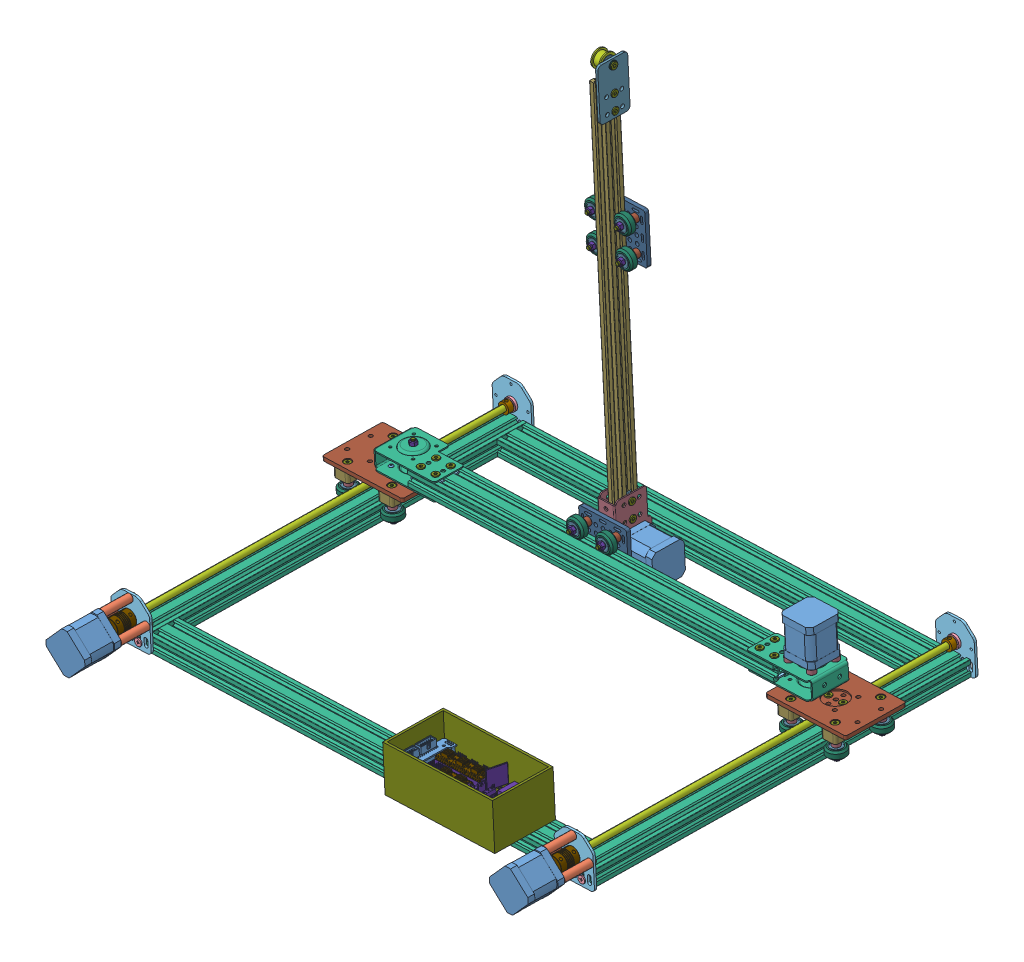
SolidWorks assembly manipulator2, configuration 預設. Lengths in mm. (continued)
Components (placement in the parent): (continued)
- Y-1: Y [Default] at (-55.2828 466.9625 1561.8962) x (0.061515 -0.998106 -0.000537) z (0.998106 0.061515 -0.00018) size (96.36 65.23 599.86) (flexible) (continued)
  - small plate-2: small plate [預設] at (444.4195 1082.4526 226.1786) x (0.999761 -0.019668 -0.009529) z (0.009662 0.00665 0.999931) size (65.63 34.48 65.67) (continued)
    - small wheel-5: small wheel [預設] at (-0.6906 23.95 24.7704) x (-0.019681 0.99952 0.023908) z (0.000235 -0.023908 0.999714) size (11 23.9 23.9) (continued)
      - Ball Bearing 5 x 16 x 5-2: Ball Bearing 5 x 16 x 5 [Default] at (-5.0567 -11.3534 -2.7479) size (5 16 16)
      - Solid V Wheel-2: Solid V Wheel [Default] at (-8.0567 -11.3534 -2.7479) size (10.2 23.9 23.9)
      - Ball Bearing 5 x 16 x 5-3: Ball Bearing 5 x 16 x 5 [Default] at (-11.0567 -11.3534 -2.7479) size (5 16 16)
    - small wheel-6: small wheel [預設] at (-40.6828 23.1636 24.7264) x (-0.019681 0.99952 0.023908) z (0.000235 -0.023908 0.999714) size (11 23.9 23.9)
      - Ball Bearing 5 x 16 x 5-2: Ball Bearing 5 x 16 x 5 [Default] at (-5.0567 -11.3534 -2.7479) size (5 16 16)
      - Solid V Wheel-2: Solid V Wheel [Default] at (-8.0567 -11.3534 -2.7479) size (10.2 23.9 23.9)
      - Ball Bearing 5 x 16 x 5-3: Ball Bearing 5 x 16 x 5 [Default] at (-11.0567 -11.3534 -2.7479) size (5 16 16)
    - Aluminum Spacer 9mm-1: Aluminum Spacer 9mm [Default] at (-29.3072 19.9403 61.9094) x (0.999806 0.019681 0.000235) z (-0.019681 0.99952 0.023908) size (10 10 9)
    - Aluminum Spacer 9mm-2: Aluminum Spacer 9mm [Default] at (10.6851 20.7267 61.9534) x (0.999806 0.019681 0.000235) z (-0.019681 0.99952 0.023908) size (10 10 9)
    - Aluminum Spacer 9mm-3: Aluminum Spacer 9mm [Default] at (-29.282 20.8973 21.9208) x (0.999806 0.019681 0.000235) z (-0.019681 0.99952 0.023908) size (10 10 9)
    - Aluminum Spacer 9mm-4: Aluminum Spacer 9mm [Default] at (10.7103 21.6837 21.9648) x (0.999806 0.019681 0.000235) z (-0.019681 0.99952 0.023908) size (10 10 9)
    - Low Profile Screw M5-7: Low Profile Screw M5 [M5 x 30] at (-28.9529 1.949 61.479) x (0.019681 -0.99952 -0.023908) z (0.000235 -0.023908 0.999714) size (31.62 9 9)
    - Low Profile Screw M5-8: Low Profile Screw M5 [M5 x 30] at (-28.9277 2.906 21.4905) x (0.019681 -0.99952 -0.023908) z (0.000235 -0.023908 0.999714) size (31.62 9 9)
    - Low Profile Screw M5-9: Low Profile Screw M5 [M5 x 30] at (11.0393 2.7354 61.523) x (0.019681 -0.99952 -0.023908) z (0.000235 -0.023908 0.999714) size (31.62 9 9)
    - Low Profile Screw M5-10: Low Profile Screw M5 [M5 x 30] at (11.0645 3.6924 21.5345) x (0.019681 -0.99952 -0.023908) z (0.000235 -0.023908 0.999714) size (31.62 9 9)
    - Nylon Insert Lock Nut M5-6: Nylon Insert Lock Nut M5 [Default] at (-29.0655 9.9026 21.6579) x (0.192329 -0.019681 0.981133) z (0.981133 0.023908 -0.191849) size (8 5 9.24)
    - Nylon Insert Lock Nut M5-7: Nylon Insert Lock Nut M5 [Default] at (-29.0907 8.9456 61.6464) x (0.192329 -0.019681 0.981133) z (0.981133 0.023908 -0.191849) size (8 5 9.24)
    - Nylon Insert Lock Nut M5-9: Nylon Insert Lock Nut M5 [Default] at (10.9016 9.732 61.6904) x (0.192329 -0.019681 0.981133) z (0.981133 0.023908 -0.191849) size (8 5 9.24)
    - Nylon Insert Lock Nut M5-10: Nylon Insert Lock Nut M5 [Default] at (10.9268 10.689 21.7018) x (0.192329 -0.019681 0.981133) z (0.981133 0.023908 -0.191849) size (8 5 9.24)
- X-1: X [Default] at (377.0186 755.9985 711.7917) x (-0.998451 -0.05295 -0.017075) z (0.052967 -0.998596 -0.000534) size (92.45 47.68 584.07) (flexible)
  - Double Tee Nut-1: Double Tee Nut [Default] at (171.529 282.1788 684.0965) x (0 0 -1) z (1 0 0) size (36.88 10 3)
  - Double Tee Nut-2: Double Tee Nut [Default] at (171.529 282.1788 220.9765) x (0 0 -1) z (1 0 0) size (36.88 10 3)
  - Low Profile Screw M5-13: Low Profile Screw M5 [M5 x 25] at (190.729 287.1788 160.7465) size (26.62 9 9)
  - Nylon Insert Lock Nut M5-4: Nylon Insert Lock Nut M5 [Default] at (185.829 287.1788 160.7465) x (0 -1 0) z (0 0 1) size (8 5 9.24)
  - Low Profile Screw M5-14: Low Profile Screw M5 [M5 x 8] at (174.729 287.1788 192.5365) size (9.62 9 9)
  - Low Profile Screw M5-15: Low Profile Screw M5 [M5 x 8] at (174.729 287.1788 212.5365) size (9.62 9 9)
  - Button Head Socket Cap Screw M3-1: Button Head Socket Cap Screw M3 [M3 x 8] at (161.729 302.6788 691.1565) x (-1 0 0) z (0 0.924225 0.381849) size (9.72 5.7 5.7)
  - Button Head Socket Cap Screw M3-3: Button Head Socket Cap Screw M3 [M3 x 8] at (161.729 302.6788 722.1565) x (-1 0 0) z (0 0.924225 0.381849) size (9.72 5.7 5.7)
  - Button Head Socket Cap Screw M3-4: Button Head Socket Cap Screw M3 [M3 x 8] at (161.729 271.6788 722.1565) x (-1 0 0) z (0 0.924225 0.381849) size (9.72 5.7 5.7)
  - Button Head Socket Cap Screw M3-5: Button Head Socket Cap Screw M3 [M3 x 8] at (161.729 271.6788 691.1565) x (-1 0 0) z (0 0.924225 0.381849) size (9.72 5.7 5.7)
  - Low Profile Screw M5-16: Low Profile Screw M5 [M5 x 8] at (176.129 287.1788 655.6565) size (9.62 9 9)
  - Low Profile Screw M5-17: Low Profile Screw M5 [M5 x 8] at (176.129 287.1788 675.6565) size (9.62 9 9)
  - Low Profile Screw M5-18: Low Profile Screw M5 [M5 x 8] at (183.329 287.1788 675.6565) x (-1 0 0) z (0 0.924225 0.381849) size (9.62 9 9)
  - Low Profile Screw M5-19: Low Profile Screw M5 [M5 x 8] at (183.329 287.1788 655.6565) x (-1 0 0) z (0 0.924225 0.381849) size (9.62 9 9)
  - Nema 17 Stepper Motor-1: Nema 17 Stepper Motor [Default] at (168.129 287.1788 706.6565) x (0 0 -1) z (1 0 0) size (42.42 42.42 72)
  - GT2 Timing Pulley 30 Tooth-1: GT2 Timing Pulley 30 Tooth [Default] at (191.729 287.1788 706.6565) x (-1 0 0) z (0 0.993409 -0.11462) size (17.5 22 22)
  - Smooth Idler-1: Smooth Idler [Default] at (179.279 287.1788 160.7465) x (-1 0 0) z (0 0.430653 -0.902518) size (13.1 22 22)
    - Smooth Idler Pulley Wheel-1: Smooth Idler Pulley Wheel [Default] at origin size (12.7 22 22)
    - Ball Bearing 5 x 16 x 5-1: Ball Bearing 5 x 16 x 5 [Default] at (4.05 0 0) x (1 0 0) z (0 0.954651 0.297727) size (5 16 16)
    - Ball Bearing 5 x 16 x 5-2: Ball Bearing 5 x 16 x 5 [Default] at (-4.05 0 0) x (1 0 0) z (0 0.976216 -0.216802) size (5 16 16)
    - Nylon Spacer 0.125in-1: Nylon Spacer 0.125in [Default] at (-1.625 0 0) x (0 -0.24187 -0.970309) z (0 -0.970309 0.24187) size (7.94 3.17 7.94)
  - V-Slot 20x20x500 Linear Rail-1: V-Slot 20x20x500 Linear Rail [Default] at (179.729 287.1788 184.0965) size (20 20 500)
  - small plate-1: small plate [預設] at (188.6703 270.6911 316.0744) x (0.999806 -0.019681 -0.000629) z (0.0011 0.023908 0.999714) size (65.63 34.48 65.67)
    - small wheel-3: small wheel [預設] at (-0.7158 22.993 64.759) x (-0.019681 0.99952 0.023908) z (0.000235 -0.023908 0.999714) size (11 23.9 23.9)
      - Ball Bearing 5 x 16 x 5-2: Ball Bearing 5 x 16 x 5 [Default] at (-5.0567 -11.3534 -2.7479) size (5 16 16)
      - Solid V Wheel-2: Solid V Wheel [Default] at (-8.0567 -11.3534 -2.7479) size (10.2 23.9 23.9)
      - Ball Bearing 5 x 16 x 5-3: Ball Bearing 5 x 16 x 5 [Default] at (-11.0567 -11.3534 -2.7479) size (5 16 16)
    - small wheel-4: small wheel [預設] at (-40.708 22.2066 64.715) x (-0.019681 0.99952 0.023908) z (0.000235 -0.023908 0.999714) size (11 23.9 23.9)
      - Ball Bearing 5 x 16 x 5-2: Ball Bearing 5 x 16 x 5 [Default] at (-5.0567 -11.3534 -2.7479) size (5 16 16)
      - Solid V Wheel-2: Solid V Wheel [Default] at (-8.0567 -11.3534 -2.7479) size (10.2 23.9 23.9)
      - Ball Bearing 5 x 16 x 5-3: Ball Bearing 5 x 16 x 5 [Default] at (-11.0567 -11.3534 -2.7479) size (5 16 16)
    - V-Slot Gantry Plate 20mm 2-1: V-Slot Gantry Plate 20mm 2 [Default] at (-9.4756 29.8077 42.1523) x (0.999806 0.01966 0.0011) z (-0.000629 -0.023925 0.999714) size (65.5 5 65.5)
    - small wheel-5: small wheel [預設] at (-0.6906 23.95 24.7704) x (-0.019681 0.99952 0.023908) z (0.000235 -0.023908 0.999714) size (11 23.9 23.9)
      - Ball Bearing 5 x 16 x 5-2: Ball Bearing 5 x 16 x 5 [Default] at (-5.0567 -11.3534 -2.7479) size (5 16 16)
      - Solid V Wheel-2: Solid V Wheel [Default] at (-8.0567 -11.3534 -2.7479) size (10.2 23.9 23.9)
      - Ball Bearing 5 x 16 x 5-3: Ball Bearing 5 x 16 x 5 [Default] at (-11.0567 -11.3534 -2.7479) size (5 16 16)
    - small wheel-6: small wheel [預設] at (-40.6828 23.1636 24.7264) x (-0.019681 0.99952 0.023908) z (0.000235 -0.023908 0.999714) size (11 23.9 23.9)
      - Ball Bearing 5 x 16 x 5-2: Ball Bearing 5 x 16 x 5 [Default] at (-5.0567 -11.3534 -2.7479) size (5 16 16)
      - Solid V Wheel-2: Solid V Wheel [Default] at (-8.0567 -11.3534 -2.7479) size (10.2 23.9 23.9)
      - Ball Bearing 5 x 16 x 5-3: Ball Bearing 5 x 16 x 5 [Default] at (-11.0567 -11.3534 -2.7479) size (5 16 16)
    - Aluminum Spacer 9mm-1: Aluminum Spacer 9mm [Default] at (-29.3072 19.9403 61.9094) x (0.999806 0.019681 0.000235) z (-0.019681 0.99952 0.023908) size (10 10 9)
    - Aluminum Spacer 9mm-2: Aluminum Spacer 9mm [Default] at (10.6851 20.7267 61.9534) x (0.999806 0.019681 0.000235) z (-0.019681 0.99952 0.023908) size (10 10 9)
    - Aluminum Spacer 9mm-3: Aluminum Spacer 9mm [Default] at (-29.282 20.8973 21.9208) x (0.999806 0.019681 0.000235) z (-0.019681 0.99952 0.023908) size (10 10 9)
    - Aluminum Spacer 9mm-4: Aluminum Spacer 9mm [Default] at (10.7103 21.6837 21.9648) x (0.999806 0.019681 0.000235) z (-0.019681 0.99952 0.023908) size (10 10 9)
    - Low Profile Screw M5-7: Low Profile Screw M5 [M5 x 30] at (-28.9529 1.949 61.479) x (0.019681 -0.99952 -0.023908) z (0.000235 -0.023908 0.999714) size (31.62 9 9)
    - Low Profile Screw M5-8: Low Profile Screw M5 [M5 x 30] at (-28.9277 2.906 21.4905) x (0.019681 -0.99952 -0.023908) z (0.000235 -0.023908 0.999714) size (31.62 9 9)
    - Low Profile Screw M5-9: Low Profile Screw M5 [M5 x 30] at (11.0393 2.7354 61.523) x (0.019681 -0.99952 -0.023908) z (0.000235 -0.023908 0.999714) size (31.62 9 9)
    - Low Profile Screw M5-10: Low Profile Screw M5 [M5 x 30] at (11.0645 3.6924 21.5345) x (0.019681 -0.99952 -0.023908) z (0.000235 -0.023908 0.999714) size (31.62 9 9)
    - Nylon Insert Lock Nut M5-6: Nylon Insert Lock Nut M5 [Default] at (-29.0655 9.9026 21.6579) x (0.192329 -0.019681 0.981133) z (0.981133 0.023908 -0.191849) size (8 5 9.24)
    - Nylon Insert Lock Nut M5-7: Nylon Insert Lock Nut M5 [Default] at (-29.0907 8.9456 61.6464) x (0.192329 -0.019681 0.981133) z (0.981133 0.023908 -0.191849) size (8 5 9.24)
    - Nylon Insert Lock Nut M5-9: Nylon Insert Lock Nut M5 [Default] at (10.9016 9.732 61.6904) x (0.192329 -0.019681 0.981133) z (0.981133 0.023908 -0.191849) size (8 5 9.24)
    - Nylon Insert Lock Nut M5-10: Nylon Insert Lock Nut M5 [Default] at (10.9268 10.689 21.7018) x (0.192329 -0.019681 0.981133) z (0.981133 0.023908 -0.191849) size (8 5 9.24)
  - Actuator End Mount 2-2: Actuator End Mount 2 [Default] at (149.1255 264.4939 741.9647) x (0 0 1) z (0 1 0) size (83 23.2 47.68)
  - Idler Pulley Plate-1: Idler Pulley Plate [Default] at (169.729 287.1788 187.2465) x (0 1 0) z (0 0 1) size (39.5 3 67)
  - Aluminum Spacer 3mm-8: Aluminum Spacer 3mm [Default] at (169.729 287.1788 160.7465) x (0 0 -1) z (1 0 0) size (10 10 3)
  - Precision Shim 10 x 5 x 1-3: Precision Shim 10 x 5 x 1 [Default] at (166.729 287.1788 160.7465) x (0 1 0) z (0 0 1) size (10 1 10)
  - Double Tee Nut-3: Double Tee Nut [Default] at (187.929 282.1788 647.2165) x (0 0 1) z (-1 0 0) size (36.88 10 3)
- arm_control-1: arm_control [預設] at (345.393 13.2248 848.7276) x (0.998451 0.05295 0.017075) z (-0.052967 0.998596 0.000534) size (150 80 60)
  - arm_control_box-1: arm_control_box [預設] at origin size (150 80 60)
  - Assembly Arduino Mega RAMPS 1.4-1: Assembly Arduino Mega RAMPS 1.4 [預設] at (65.2821 38.0889 23) x (0 1 0) z (0 0 1) size (61.87 117.14 43.8)
    - User Library-MF-R500___ _________-1: User Library-MF-R500___ _________ [預設] at origin size (61.76 111.7 43.8)
    - Heatsink For A4988-1: Heatsink For A4988 [預設] at (12.2453 -11.1934 10.806) size (15.24 20.32 16.04)
    - Heatsink For A4988-2: Heatsink For A4988 [預設] at (12.2453 9.2066 10.806) size (15.24 20.32 16.04)
    - Heatsink For A4988-3: Heatsink For A4988 [預設] at (12.2453 29.6066 10.806) size (15.24 20.32 16.04)
    - Heatsink For A4988-4: Heatsink For A4988 [預設] at (-10.8547 -11.1934 10.806) size (15.24 20.32 16.04)
    - Heatsink For A4988-5: Heatsink For A4988 [預設] at (-10.8547 9.2066 10.806) size (15.24 20.32 16.04)
    - PCB_LCD-1: PCB_LCD [預設] at (1.0941 49.1719 11.077) size (60.45 19.63 19.5)
Mates (geometry in assembly coordinates):
- 重合/共線/共點2: coincident: point of Z2-1/V-Slot 20x40x500 Linear Rail-1; point of V-Slot 20x40x500 Linear Rail-1
- 重合/共線/共點3: coincident: point of Z2-1/V-Slot 20x40x500 Linear Rail-1; point of V-Slot 20x40x500 Linear Rail-1
- 重合/共線/共點4: coincident anti-aligned: plane of Z2-1/V-Slot 20x40x500 Linear Rail-1 through (-18.821 -16.0825 801.9787) normal (0.998451 0.05295 0.017075); plane of V-Slot 20x40x500 Linear Rail-1 through (-10.6501 -15.3924 322.0487) normal (-0.998451 -0.05295 -0.017075)
- 同軸心6: concentric anti-aligned: cylinder of Z2-1/mid plate-3/V-Slot Gantry Plate 20-80mm 2-1 through (11.2704 19.182 444.0234) axis (0.052967 -0.998596 -0.000534) radius 2.55; cone of Aluminum Spacer 3mm-1 through (11.2598 19.3817 444.0235) axis (-0.052967 0.998596 0.000534)
- 重合/共線/共點11: coincident anti-aligned: plane of Z2-1/mid plate-3/V-Slot Gantry Plate 20-80mm 2-1 through (-87.2718 13.9281 494.8458) normal (-0.052967 0.998596 0.000534); plane of Aluminum Spacer 3mm-1 through (11.2704 19.182 444.0234) normal (0.052967 -0.998596 -0.000534)
- 同軸心7: concentric anti-aligned: cylinder of Z2-1/mid plate-3/V-Slot Gantry Plate 20-80mm 2-1 through (-19.6816 17.5406 443.4941) axis (0.052967 -0.998596 -0.000534) radius 2.55; cone of Aluminum Spacer 3mm-2 through (-19.6922 17.7403 443.4942) axis (-0.052967 0.998596 0.000534)
- 重合/共線/共點12: coincident anti-aligned: plane of Z2-1/mid plate-3/V-Slot Gantry Plate 20-80mm 2-1 through (-87.2718 13.9281 494.8458) normal (-0.052967 0.998596 0.000534); plane of Aluminum Spacer 3mm-2 through (-19.6816 17.5406 443.4941) normal (0.052967 -0.998596 -0.000534)
- 同軸心8: concentric anti-aligned: cylinder of Z2-1/mid plate-3/V-Slot Gantry Plate 20-80mm 2-1 through (-20.2093 17.496 474.4896) axis (0.052967 -0.998596 -0.000534) radius 2.55; cone of Aluminum Spacer 3mm-3 through (-20.2199 17.6957 474.4897) axis (-0.052967 0.998596 0.000534)
- 重合/共線/共點13: coincident anti-aligned: plane of Z2-1/mid plate-3/V-Slot Gantry Plate 20-80mm 2-1 through (-87.2718 13.9281 494.8458) normal (-0.052967 0.998596 0.000534); plane of Aluminum Spacer 3mm-3 through (-20.2093 17.496 474.4896) normal (0.052967 -0.998596 -0.000534)
- 同軸心9: concentric anti-aligned: cylinder of Z2-1/mid plate-3/V-Slot Gantry Plate 20-80mm 2-1 through (10.7427 19.1375 475.0189) axis (0.052967 -0.998596 -0.000534) radius 2.55; cone of Aluminum Spacer 3mm-4 through (10.7321 19.3372 475.019) axis (-0.052967 0.998596 0.000534)
- 重合/共線/共點14: coincident anti-aligned: plane of Z2-1/mid plate-3/V-Slot Gantry Plate 20-80mm 2-1 through (-87.2718 13.9281 494.8458) normal (-0.052967 0.998596 0.000534); plane of Aluminum Spacer 3mm-4 through (10.7427 19.1375 475.0189) normal (0.052967 -0.998596 -0.000534)
- 重合/共線/共點15: coincident anti-aligned: plane of Y-1/Linear Actuator End Mount-2 through (-95.6831 19.5216 436.4021) normal (0.052967 -0.998596 -0.000534); plane of Aluminum Spacer 3mm-2 through (-19.9994 23.5322 443.4973) normal (-0.052967 0.998596 0.000534)
- 同軸心10: concentric anti-aligned: cylinder of Z2-1/mid plate-3/V-Slot Gantry Plate 20-80mm 2-1 through (-19.6816 17.5406 443.4941) axis (0.052967 -0.998596 -0.000534) radius 2.55; cylinder of Y-1/Linear Actuator End Mount-2 through (-20.0841 25.1299 443.4981) axis (-0.052967 0.998596 0.000534) radius 1.8
- 同軸心11: concentric anti-aligned: cylinder of Z2-1/mid plate-3/V-Slot Gantry Plate 20-80mm 2-1 through (11.2704 19.182 444.0234) axis (0.052967 -0.998596 -0.000534) radius 2.55; cylinder of Y-1/Linear Actuator End Mount-2 through (10.8679 26.7714 444.0275) axis (-0.052967 0.998596 0.000534) radius 1.8
- 同軸心12: concentric aligned: cylinder of Y-1/Linear Actuator End Mount-2 through (-20.0841 25.1299 443.4981) axis (-0.052967 0.998596 0.000534) radius 1.8; cylinder of Button Head Socket Cap Screw M3-1 through (-20.0841 25.1299 443.4981) axis (-0.052967 0.998596 0.000534) radius 2.85
- 重合/共線/共點16: coincident anti-aligned: plane of Y-1/Linear Actuator End Mount-2 through (-95.7678 21.1194 436.403) normal (-0.052967 0.998596 0.000534); plane of Button Head Socket Cap Screw M3-1 through (-17.2381 25.2809 443.4967) normal (0.052967 -0.998596 -0.000534)
- 同軸心13: concentric aligned: cylinder of Y-1/Linear Actuator End Mount-2 through (10.8679 26.7714 444.0275) axis (-0.052967 0.998596 0.000534) radius 1.8; cylinder of Button Head Socket Cap Screw M3-2 through (10.8679 26.7714 444.0275) axis (-0.052967 0.998596 0.000534) radius 2.85
- 重合/共線/共點17: coincident anti-aligned: plane of Y-1/Linear Actuator End Mount-2 through (-95.7678 21.1194 436.403) normal (-0.052967 0.998596 0.000534); plane of Button Head Socket Cap Screw M3-2 through (13.7138 26.9223 444.026) normal (0.052967 -0.998596 -0.000534)
- 同軸心14: concentric aligned: cylinder of Y-1/Linear Actuator End Mount-2 through (-20.6118 25.0854 474.4936) axis (-0.052967 0.998596 0.000534) radius 1.8; cylinder of Button Head Socket Cap Screw M3-3 through (-20.6118 25.0854 474.4936) axis (-0.052967 0.998596 0.000534) radius 2.85
- 重合/共線/共點18: coincident anti-aligned: plane of Y-1/Linear Actuator End Mount-2 through (-95.7678 21.1194 436.403) normal (-0.052967 0.998596 0.000534); plane of Button Head Socket Cap Screw M3-3 through (-17.7658 25.2363 474.4922) normal (0.052967 -0.998596 -0.000534)
- 同軸心15: concentric aligned: cylinder of Y-1/Linear Actuator End Mount-2 through (10.3401 26.7268 475.0229) axis (-0.052967 0.998596 0.000534) radius 1.8; cylinder of Button Head Socket Cap Screw M3-4 through (10.3401 26.7268 475.0229) axis (-0.052967 0.998596 0.000534) radius 2.85
- 重合/共線/共點19: coincident anti-aligned: plane of Y-1/Linear Actuator End Mount-2 through (-95.7678 21.1194 436.403) normal (-0.052967 0.998596 0.000534); plane of Button Head Socket Cap Screw M3-4 through (13.1861 26.8777 475.0215) normal (0.052967 -0.998596 -0.000534)
- 同軸心16: concentric anti-aligned: cylinder of Button Head Socket Cap Screw M3-1 through (-20.0841 25.1299 443.4981) axis (0.052967 -0.998596 -0.000534) radius 1.5; cylinder of Nylon Insert Lock Nut M3-6 through (-19.4168 12.5476 443.4914) axis (-0.052967 0.998596 0.000534) radius 1.5
- 同軸心17: concentric anti-aligned: cylinder of Button Head Socket Cap Screw M3-2 through (10.8679 26.7714 444.0275) axis (0.052967 -0.998596 -0.000534) radius 1.5; cylinder of Nylon Insert Lock Nut M3-3 through (11.5352 14.189 444.0207) axis (-0.052967 0.998596 0.000534) radius 1.5
- 同軸心18: concentric anti-aligned: cylinder of Button Head Socket Cap Screw M3-3 through (-20.6118 25.0854 474.4936) axis (0.052967 -0.998596 -0.000534) radius 1.5; cylinder of Nylon Insert Lock Nut M3-5 through (-19.9445 12.503 474.4869) axis (-0.052967 0.998596 0.000534) radius 1.5
- 同軸心19: concentric anti-aligned: cylinder of Button Head Socket Cap Screw M3-4 through (10.3401 26.7268 475.0229) axis (0.052967 -0.998596 -0.000534) radius 1.5; cylinder of Nylon Insert Lock Nut M3-4 through (11.0075 14.1445 475.0162) axis (-0.052967 0.998596 0.000534) radius 1.5
- 重合/共線/共點21: coincident anti-aligned: plane of Z2-1/mid plate-3/V-Slot Gantry Plate 20-80mm 2-1 through (-87.007 8.9351 494.8431) normal (0.052967 -0.998596 -0.000534); plane of Nylon Insert Lock Nut M3-6 through (-17.9192 12.6271 443.4612) normal (-0.052967 0.998596 0.000534)
- 重合/共線/共點22: coincident anti-aligned: plane of Z2-1/mid plate-3/V-Slot Gantry Plate 20-80mm 2-1 through (-87.007 8.9351 494.8431) normal (0.052967 -0.998596 -0.000534); plane of Nylon Insert Lock Nut M3-5 through (-18.4469 12.5825 474.4567) normal (-0.052967 0.998596 0.000534)
- 重合/共線/共點23: coincident anti-aligned: plane of Z2-1/mid plate-3/V-Slot Gantry Plate 20-80mm 2-1 through (-87.007 8.9351 494.8431) normal (0.052967 -0.998596 -0.000534); plane of Nylon Insert Lock Nut M3-4 through (12.5051 14.2239 474.986) normal (-0.052967 0.998596 0.000534)
- 重合/共線/共點24: coincident anti-aligned: plane of Z2-1/mid plate-3/V-Slot Gantry Plate 20-80mm 2-1 through (-87.007 8.9351 494.8431) normal (0.052967 -0.998596 -0.000534); plane of Nylon Insert Lock Nut M3-3 through (13.0328 14.2685 443.9905) normal (-0.052967 0.998596 0.000534)
- 平行相距1: distance = 15 mm aligned: plane of Y-1/Linear Actuator End Mount-1 through (520.06 53.7798 443.234) normal (0.017023 0.001438 -0.999854); plane of Z2-4/mid plate-3/V-Slot Gantry Plate 20-80mm 2-1 through (622.9393 51.6331 429.9803) normal (0.017023 0.001438 -0.999854)
- 同軸心20: concentric anti-aligned: cylinder of Y-1/small plate-2/V-Slot Gantry Plate 20mm 2-1 through (240.1481 28.9687 443.8836) axis (-0.017023 -0.001438 0.999854) radius 2.55; cylinder of X-1/Actuator End Mount 2-2 through (240.1754 28.971 442.2838) axis (0.017023 0.001438 -0.999854) radius 2.55
- 同軸心21: concentric anti-aligned: cylinder of Y-1/small plate-2/V-Slot Gantry Plate 20mm 2-1 through (239.6185 38.9547 443.8889) axis (-0.017023 -0.001438 0.999854) radius 2.55; cylinder of X-1/Actuator End Mount 2-2 through (239.6457 38.957 442.2891) axis (0.017023 0.001438 -0.999854) radius 2.55
- 重合/共線/共點25: coincident anti-aligned: plane of Y-1/small plate-2/V-Slot Gantry Plate 20mm 2-1 through (267.217 80.2241 444.4181) normal (0.017023 0.001438 -0.999854); plane of X-1/Actuator End Mount 2-2 through (184.8923 58.1295 442.9848) normal (-0.017023 -0.001438 0.999854)
- 重合/共線/共點26: coincident anti-aligned: plane of V-Slot 20x40x500 Linear Rail-2 through (-19.0102 -6.0678 781.987) normal (-0.052967 0.998596 0.000534); plane of arm_control-1/arm_control_box-1 through (166.2231 3.7231 845.6635) normal (0.052967 -0.998596 -0.000534)
- 重合/共線/共點27: coincident anti-aligned: line of V-Slot 20x40x500 Linear Rail-2 through (-18.6783 -6.0397 762.4898) axis (0.998451 0.05295 0.017075); line of arm_control-1/arm_control_box-1 through (317.3526 11.7806 768.2364) axis (-0.998451 -0.05295 -0.017075)
- 平行相距3: distance = 50 mm anti-aligned: plane of arm_control-1/arm_control_box-1 through (491.9827 81.0831 851.3208) normal (0.998451 0.05295 0.017075); plane of Z2-4/V-Slot 20x40x500 Linear Rail-1 through (546.3023 13.887 811.6431) normal (-0.998451 -0.05295 -0.017075)
